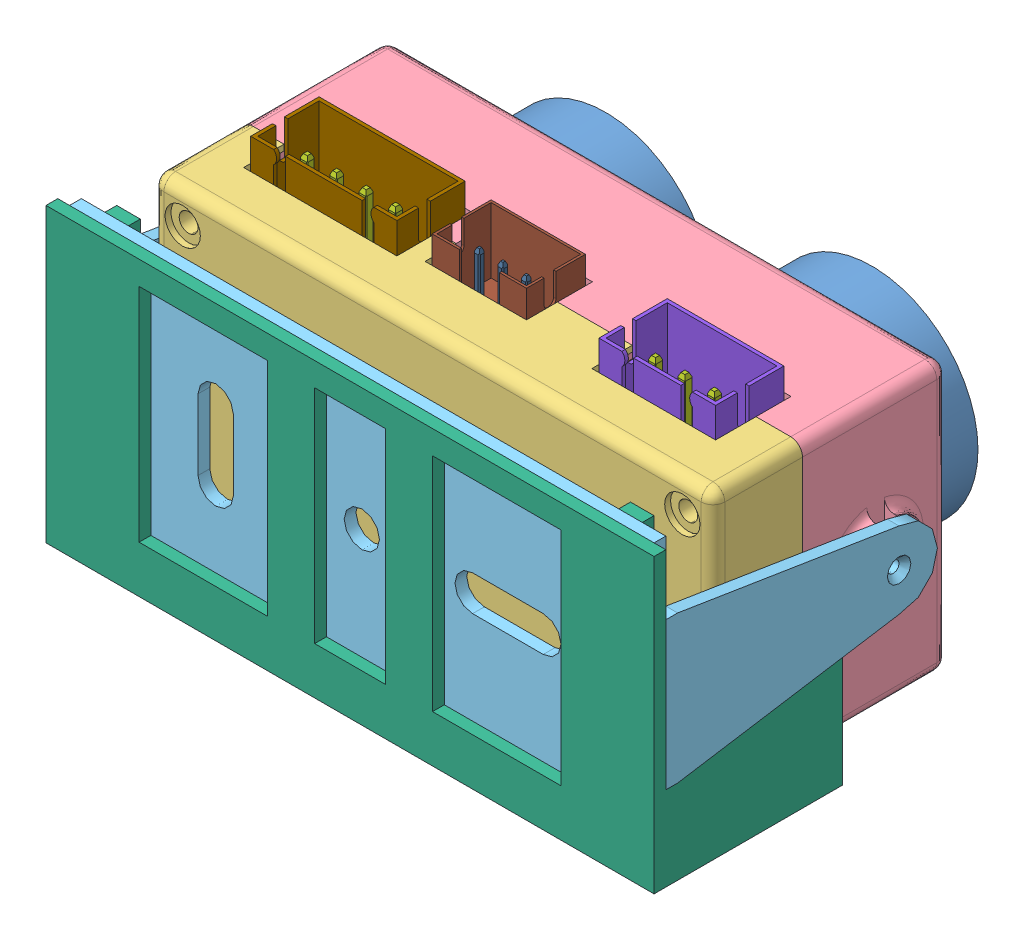
SolidWorks assembly assembly, configuration По умолчанию. Lengths in mm.
Overall size (51.6 27.1 32.99).
213 component instances, 60 part files, 18 mates.
Components (placement in the parent):
- hc-sr04-1: hc-sr04 [По умолчанию] at origin size (45.2 20.4 11.6)
- Assembly.step-1: Assembly.step [По умолчанию] at (-22.6 57.6501 -6.8032) x (1 0 0) z (0 0 1) size (47.6 23.9 18.81)
  - Assembly-asm1.step-1: Assembly-asm1.step [По умолчанию] at origin size (45.2 20.4 11.54)
    - Assembly-asm2.step-1: Assembly-asm2.step [По умолчанию] at (0 -47.4501 18.5211) x (1 0 0) z (0 0 -1) size (45.2 20.4 11.54)
      - X1.step-1: X1.step [По умолчанию] at (40.4891 10.7965 0) x (0 -1 0) z (0 0 1) size (10.16 2.54 11.54)
        - PLS-4.step-1: PLS-4.step [По умолчанию] at origin size (10.16 2.54 11.54)
          - PLS-1.step-1: PLS-1.step [По умолчанию] at (-1.27 0 0) size (2.54 2.54 11.54)
            - ____________.step-1: ____________.step [По умолчанию] at (0 0 -3) size (0.64 0.64 11.54)
            - _________.step-1: _________.step [По умолчанию] at origin size (2.54 2.54 2.54)
          - PLS-1.step-2: PLS-1.step [По умолчанию] at (-1.27 0 0) size (2.54 2.54 11.54)
            - ____________.step-1: ____________.step [По умолчанию] at (0 0 -3) size (0.64 0.64 11.54)
            - _________.step-1: _________.step [По умолчанию] at origin size (2.54 2.54 2.54)
          - PLS-1.step-3: PLS-1.step [По умолчанию] at (-3.81 0 0) size (2.54 2.54 11.54)
            - ____________.step-1: ____________.step [По умолчанию] at (0 0 -3) size (0.64 0.64 11.54)
            - _________.step-1: _________.step [По умолчанию] at origin size (2.54 2.54 2.54)
          - PLS-1.step-4: PLS-1.step [По умолчанию] at (1.27 0 0) size (2.54 2.54 11.54)
            - ____________.step-1: ____________.step [По умолчанию] at (0 0 -3) size (0.64 0.64 11.54)
            - _________.step-1: _________.step [По умолчанию] at origin size (2.54 2.54 2.54)
          - PLS-1.step-5: PLS-1.step [По умолчанию] at (3.81 0 0) size (2.54 2.54 11.54)
            - ____________.step-1: ____________.step [По умолчанию] at (0 0 -3) size (0.64 0.64 11.54)
            - _________.step-1: _________.step [По умолчанию] at origin size (2.54 2.54 2.54)
      - R4.step-1: R4.step [По умолчанию] at (17.4997 9.4504 0) x (1 0 0) z (0 0 1) size (1 0.51 0.35)
        - r0402.step-1: r0402.step [По умолчанию] at origin size (1 0.51 0.35)
      - R3.step-1: R3.step [По умолчанию] at (17.4997 6.8046 0) x (1 0 0) z (0 0 1) size (1 0.51 0.35)
        - r0402-0.step-1: r0402-0.step [По умолчанию] at origin size (1 0.51 0.35)
      - R2.step-1: R2.step [По умолчанию] at (17.4997 10.7046 0) x (-1 0 0) z (0 0 1) size (1 0.51 0.35)
        - r0402-1.step-1: r0402-1.step [По умолчанию] at origin size (1 0.51 0.35)
      - R1.step-1: R1.step [По умолчанию] at (17.4997 5.5504 0) x (-1 0 0) z (0 0 1) size (1 0.51 0.35)
        - r0402-2.step-1: r0402-2.step [По умолчанию] at origin size (1 0.51 0.35)
      - L1.step-1: L1.step [По умолчанию] at (32.2997 12.4504 0) x (0 -1 0) z (0 0 1) size (10.63 10.22 3.88)
        - Combine1.step-1: Combine1.step [По умолчанию] at origin size (10.63 10.22 3.88)
      - D1.step-1: D1.step [По умолчанию] at (23.1002 6.1507 0) x (-1 0 0) z (0 0 1) size (6 4.9 1.75)
        - User Library-SOIC-8-1.step-1: User Library-SOIC-8-1.step [По умолчанию] at origin size (6 4.9 1.75)
      - C7.step-1: C7.step [По умолчанию] at (17.4997 8.0804 0) x (-1 0 0) z (0 0 1) size (1 0.5 0.5)
        - User Library-Capacitor 0402.step-1: User Library-Capacitor 0402.step [По умолчанию] at origin size (1 0.5 0.5)
      - C6.step-1: C6.step [По умолчанию] at (17.4997 4.2457 0) x (1 0 0) z (0 0 1) size (1 0.5 0.5)
        - User Library-Capacitor 0402-3.step-1: User Library-Capacitor 0402-3.step [По умолчанию] at origin size (1 0.5 0.5)
      - C5.step-1: C5.step [По умолчанию] at (24.7543 14.1504 0) x (0 1 0) z (0 0 1) size (4 2.49 1.7)
        - User Library-1210(3225M) Cap.step-1: User Library-1210(3225M) Cap.step [По умолчанию] at origin size (4 2.49 1.7)
      - C4.step-1: C4.step [По умолчанию] at (21.2 14.15 0) x (0 1 0) z (0 0 1) size (4 2.49 1.7)
        - User Library-1210(3225M) Cap-4.step-1: User Library-1210(3225M) Cap-4.step [По умолчанию] at origin size (4 2.49 1.7)
      - C3.step-1: C3.step [По умолчанию] at (28.8 3.2 0) x (0 1 0) z (0 0 1) size (4 2.49 1.7)
        - User Library-1210(3225M) Cap-5.step-1: User Library-1210(3225M) Cap-5.step [По умолчанию] at origin size (4 2.49 1.7)
      - C2.step-1: C2.step [По умолчанию] at (17.4997 11.9589 0) x (-1 0 0) z (0 0 1) size (1 0.5 0.5)
        - User Library-Capacitor 0402-6.step-1: User Library-Capacitor 0402-6.step [По умолчанию] at origin size (1 0.5 0.5)
      - C1.step-1: C1.step [По умолчанию] at (33.9 4.9 0) x (0 -1 0) z (0 0 1) size (1 0.5 0.5)
        - User Library-Capacitor 0402-7.step-1: User Library-Capacitor 0402-7.step [По умолчанию] at origin size (1 0.5 0.5)
      - Board.step-1: Board.step [По умолчанию] at origin size (45.2 20.4 1.27)
  - Assembly-asm19.step-1: Assembly-asm19.step [По умолчанию] at origin size (47.6 23.9 18.21)
    - Assembly-asm20.step-1: Assembly-asm20.step [По умолчанию] at (0 -67.8501 12.5211) x (1 0 0) z (0 0 1) size (47.6 23.9 18.21)
      - C8.step-1: C8.step [По умолчанию] at (34.625 1.3 0) x (1 0 0) z (0 0 1) size (1 0.5 0.5)
        - User Library-Capacitor 0402-8.step-1: User Library-Capacitor 0402-8.step [По умолчанию] at origin size (1 0.5 0.5)
      - C7-1.step-1: C7-1.step [По умолчанию] at (32.625 1.3 0) x (-1 0 0) z (0 0 1) size (1 0.5 0.5)
        - User Library-Capacitor 0402-9.step-1: User Library-Capacitor 0402-9.step [По умолчанию] at origin size (1 0.5 0.5)
      - D4.step-1: D4.step [По умолчанию] at (33.625 4.8 0) x (0 1 0) z (0 0 1) size (4.3 4.5 1.51)
        - SW3dPS-SOT-89-1.step-1: SW3dPS-SOT-89-1.step [По умолчанию] at origin size (4.3 4.5 1.51)
      - X5.step-1: X5.step [По умолчанию] at (40.5 9.6 0) x (0 1 0) z (0 0 1) size (10.16 2.54 11.6)
        - User Library-PBS-04.step-1: User Library-PBS-04.step [По умолчанию] at origin size (10.16 2.54 11.6)
      - X6.step-1: X6.step [По умолчанию] at (24.1 1.9 0) x (-1 0 0) z (0 0 1) size (10.16 2.54 11.54)
        - PLS-4-1.step-1: PLS-4-1.step [По умолчанию] at origin size (10.16 2.54 11.54)
          - PLS-1.step-1: PLS-1.step [По умолчанию] at (-1.27 0 -1.2711) x (1 0 0) z (0 0 -1) size (2.54 2.54 11.54)
            - ____________.step-1: ____________.step [По умолчанию] at (0 0 -3) size (0.64 0.64 11.54)
            - _________.step-1: _________.step [По умолчанию] at origin size (2.54 2.54 2.54)
          - PLS-1.step-2: PLS-1.step [По умолчанию] at (-1.27 0 -1.2711) x (1 0 0) z (0 0 -1) size (2.54 2.54 11.54)
            - ____________.step-1: ____________.step [По умолчанию] at (0 0 -3) size (0.64 0.64 11.54)
            - _________.step-1: _________.step [По умолчанию] at origin size (2.54 2.54 2.54)
          - PLS-1.step-3: PLS-1.step [По умолчанию] at (-3.81 0 -1.2711) x (1 0 0) z (0 0 -1) size (2.54 2.54 11.54)
            - ____________.step-1: ____________.step [По умолчанию] at (0 0 -3) size (0.64 0.64 11.54)
            - _________.step-1: _________.step [По умолчанию] at origin size (2.54 2.54 2.54)
          - PLS-1.step-4: PLS-1.step [По умолчанию] at (1.27 0 -1.2711) x (1 0 0) z (0 0 -1) size (2.54 2.54 11.54)
            - ____________.step-1: ____________.step [По умолчанию] at (0 0 -3) size (0.64 0.64 11.54)
            - _________.step-1: _________.step [По умолчанию] at origin size (2.54 2.54 2.54)
          - PLS-1.step-5: PLS-1.step [По умолчанию] at (3.81 0 -1.2711) x (1 0 0) z (0 0 -1) size (2.54 2.54 11.54)
            - ____________.step-1: ____________.step [По умолчанию] at (0 0 -3) size (0.64 0.64 11.54)
            - _________.step-1: _________.step [По умолчанию] at origin size (2.54 2.54 2.54)
      - R1-1.step-1: R1-1.step [По умолчанию] at (6.2454 5.85 0) x (-1 0 0) z (0 0 1) size (1 0.51 0.35)
        - r0402-10.step-1: r0402-10.step [По умолчанию] at origin size (1 0.51 0.35)
      - C2-1.step-1: C2-1.step [По умолчанию] at (6.2454 2.35 0) x (1 0 0) z (0 0 1) size (1 0.5 0.5)
        - User Library-Capacitor 0402-11.step-1: User Library-Capacitor 0402-11.step [По умолчанию] at origin size (1 0.5 0.5)
      - C1-1.step-1: C1-1.step [По умолчанию] at (6.2454 4.817 0) x (1 0 0) z (0 0 1) size (1 0.5 0.5)
        - User Library-Capacitor 0402-12.step-1: User Library-Capacitor 0402-12.step [По умолчанию] at origin size (1 0.5 0.5)
      - X4.step-1: X4.step [По умолчанию] at (37.2 16.6 0) x (1 0 0) z (0 0 1) size (9.9 7.54 9.15)
        - xh-3aw.step-1: xh-3aw.step [По умолчанию] at origin size (9.9 7.54 9.15)
          - pin.step-1: pin.step [По умолчанию] at (-0.0001 0.02 -3.35) x (1 0 0) z (0 0 -1) size (0.64 6.32 7.12)
          - pin.step-2: pin.step [По умолчанию] at (-2.5001 0.02 -3.35) x (1 0 0) z (0 0 -1) size (0.64 6.32 7.12)
          - pin.step-3: pin.step [По умолчанию] at (2.4999 0.02 -3.35) x (1 0 0) z (0 0 -1) size (0.64 6.32 7.12)
          - xh-3aw-13.step-1: xh-3aw-13.step [По умолчанию] at origin size (9.9 7 5.8)
      - X3.step-1: X3.step [По умолчанию] at (8.9 16.7 0) x (1 0 0) z (0 0 1) size (12.4 7.54 9.15)
        - xh-4aw.step-1: xh-4aw.step [По умолчанию] at origin size (12.4 7.54 9.15)
          - pin.step-1: pin.step [По умолчанию] at (1.2501 -0.0199 -3.35) x (1 0 0) z (0 0 -1) size (0.64 6.32 7.12)
          - pin.step-2: pin.step [По умолчанию] at (3.7501 -0.0199 -3.35) x (1 0 0) z (0 0 -1) size (0.64 6.32 7.12)
          - pin.step-3: pin.step [По умолчанию] at (-3.7499 -0.0199 -3.35) x (1 0 0) z (0 0 -1) size (0.64 6.32 7.12)
          - pin.step-4: pin.step [По умолчанию] at (-1.2499 -0.0199 -3.35) x (1 0 0) z (0 0 -1) size (0.64 6.32 7.12)
          - xh-4aw-14.step-1: xh-4aw-14.step [По умолчанию] at origin size (12.4 7 5.8)
      - X2.step-1: X2.step [По умолчанию] at (21.3 17.6 0) x (1 0 0) z (0 0 1) size (8 6.25 8.4)
        - ph-3aw.step-1: ph-3aw.step [По умолчанию] at origin size (8 6.25 8.4)
          - pin-15.step-1: pin-15.step [По умолчанию] at (-2.0001 0.0249 -3.4) x (1 0 0) z (0 0 -1) size (0.5 5.25 6.65)
          - pin-15.step-2: pin-15.step [По умолчанию] at (1.9999 0.0249 -3.4) x (1 0 0) z (0 0 -1) size (0.5 5.25 6.65)
          - pin-15.step-3: pin-15.step [По умолчанию] at (-0.0001 0.0249 -3.4) x (1 0 0) z (0 0 -1) size (0.5 5.25 6.65)
          - ph-3aw-16.step-1: ph-3aw-16.step [По умолчанию] at origin size (8 6 5)
      - X1-1.step-1: X1-1.step [По умолчанию] at (3.5 5.835 0) x (0 1 0) z (0 0 1) size (5.08 6.09 4.74)
        - pls1.27-4R.step-1: pls1.27-4R.step [По умолчанию] at origin size (5.08 6.09 4.74)
          - housing.step-1: housing.step [По умолчанию] at (1.8951 0.5051 1.27) x (-1 0 0) z (0 1 0) size (1.27 2.4 1.5)
          - housing.step-2: housing.step [По умолчанию] at (-1.9149 0.5051 1.27) x (-1 0 0) z (0 1 0) size (1.27 2.4 1.5)
          - housing.step-3: housing.step [По умолчанию] at (-0.6449 0.5051 1.27) x (-1 0 0) z (0 1 0) size (1.27 2.4 1.5)
          - housing.step-4: housing.step [По умолчанию] at (0.6251 0.5051 1.27) x (-1 0 0) z (0 1 0) size (1.27 2.4 1.5)
          - pin-17.step-1: pin-17.step [По умолчанию] at (-0.6449 5.8951 1.27) x (-1 0 0) z (0 1 0) size (0.4 3.74 6.09)
          - pin-17.step-2: pin-17.step [По умолчанию] at (-1.9149 5.8951 1.27) x (-1 0 0) z (0 1 0) size (0.4 3.74 6.09)
          - pin-17.step-3: pin-17.step [По умолчанию] at (0.6251 5.8951 1.27) x (-1 0 0) z (0 1 0) size (0.4 3.74 6.09)
          - pin-17.step-4: pin-17.step [По умолчанию] at (1.8951 5.8951 1.27) x (-1 0 0) z (0 1 0) size (0.4 3.74 6.09)
      - VT3.step-1: VT3.step [По умолчанию] at (14.3043 13.2 0) x (0 1 0) z (0 0 1) size (2.64 3.05 1.12)
        - SOT95P237X112-3N.step.step-1: SOT95P237X112-3N.step.step [По умолчанию] at origin size (2.64 3.05 1.12)
          - Open CASCADE STEP translator 6.8 8.1.1.step-1: Open CASCADE STEP translator 6.8 8.1.1.step [По умолчанию] at (-0.7 -1.52 0) size (1.41 3.05 1.11)
          - Leader.step-1: Leader.step [По умолчанию] at (-0.7 -0.95 0) x (-1 0 0) z (0 0 1) size (0.62 0.5 0.61)
          - Leader.step-2: Leader.step [По умолчанию] at (-0.7 0.95 0) x (-1 0 0) z (0 0 1) size (0.62 0.5 0.61)
          - Leader.step-3: Leader.step [По умолчанию] at (0.7 0 0) size (0.62 0.5 0.61)
      - VT2.step-1: VT2.step [По умолчанию] at (10.2 13.2 0) x (0 1 0) z (0 0 1) size (2.64 3.05 1.12)
        - SOT95P237X112-3N.step-1.step-1: SOT95P237X112-3N.step-1.step [По умолчанию] at origin size (2.64 3.05 1.12)
          - Open CASCADE STEP translator 6.8 8.1.1.step-1: Open CASCADE STEP translator 6.8 8.1.1.step [По умолчанию] at (-0.7 -1.52 0) size (1.41 3.05 1.11)
          - Leader.step-1: Leader.step [По умолчанию] at (-0.7 -0.95 0) x (-1 0 0) z (0 0 1) size (0.62 0.5 0.61)
          - Leader.step-2: Leader.step [По умолчанию] at (-0.7 0.95 0) x (-1 0 0) z (0 0 1) size (0.62 0.5 0.61)
          - Leader.step-3: Leader.step [По умолчанию] at (0.7 0 0) size (0.62 0.5 0.61)
      - VT1.step-1: VT1.step [По умолчанию] at (6.0957 13.2 0) x (0 1 0) z (0 0 1) size (2.64 3.05 1.12)
        - SOT95P237X112-3N.step-2.step-1: SOT95P237X112-3N.step-2.step [По умолчанию] at origin size (2.64 3.05 1.12)
          - Open CASCADE STEP translator 6.8 8.1.1.step-1: Open CASCADE STEP translator 6.8 8.1.1.step [По умолчанию] at (-0.7 -1.52 0) size (1.41 3.05 1.11)
          - Leader.step-1: Leader.step [По умолчанию] at (-0.7 -0.95 0) x (-1 0 0) z (0 0 1) size (0.62 0.5 0.61)
          - Leader.step-2: Leader.step [По умолчанию] at (-0.7 0.95 0) x (-1 0 0) z (0 0 1) size (0.62 0.5 0.61)
          - Leader.step-3: Leader.step [По умолчанию] at (0.7 0 0) size (0.62 0.5 0.61)
      - VD1.step-1: VD1.step [По умолчанию] at (21.3 14.4 0) x (0 1 0) z (0 0 1) size (2.64 3.05 1.12)
        - SOT95P237X112-3N.step-3.step-1: SOT95P237X112-3N.step-3.step [По умолчанию] at origin size (2.64 3.05 1.12)
          - Open CASCADE STEP translator 6.8 8.1.1.step-1: Open CASCADE STEP translator 6.8 8.1.1.step [По умолчанию] at (-0.7 -1.52 0) size (1.41 3.05 1.11)
          - Leader.step-1: Leader.step [По умолчанию] at (-0.7 -0.95 0) x (-1 0 0) z (0 0 1) size (0.62 0.5 0.61)
          - Leader.step-2: Leader.step [По умолчанию] at (-0.7 0.95 0) x (-1 0 0) z (0 0 1) size (0.62 0.5 0.61)
          - Leader.step-3: Leader.step [По умолчанию] at (0.7 0 0) size (0.62 0.5 0.61)
      - R14.step-1: R14.step [По умолчанию] at (14.6085 10.0448 0) x (0 1 0) z (0 0 1) size (1 0.51 0.35)
        - r0402-18.step-1: r0402-18.step [По умолчанию] at origin size (1 0.51 0.35)
      - R13.step-1: R13.step [По умолчанию] at (13.3543 10.0448 0) x (0 1 0) z (0 0 1) size (1 0.51 0.35)
        - r0402-19.step-1: r0402-19.step [По умолчанию] at origin size (1 0.51 0.35)
      - R12.step-1: R12.step [По умолчанию] at (10.5043 10.0448 0) x (0 1 0) z (0 0 1) size (1 0.51 0.35)
        - r0402-20.step-1: r0402-20.step [По умолчанию] at origin size (1 0.51 0.35)
      - R11.step-1: R11.step [По умолчанию] at (9.25 10.0448 0) x (0 1 0) z (0 0 1) size (1 0.51 0.35)
        - r0402-21.step-1: r0402-21.step [По умолчанию] at origin size (1 0.51 0.35)
      - R10.step-1: R10.step [По умолчанию] at (6.4 10.0448 0) x (0 1 0) z (0 0 1) size (1 0.51 0.35)
        - r0402-22.step-1: r0402-22.step [По умолчанию] at origin size (1 0.51 0.35)
      - R9.step-1: R9.step [По умолчанию] at (5.1457 10.0448 0) x (0 1 0) z (0 0 1) size (1 0.51 0.35)
        - r0402-23.step-1: r0402-23.step [По умолчанию] at origin size (1 0.51 0.35)
      - R8.step-1: R8.step [По умолчанию] at (17.55 11.1 0) x (0 1 0) z (0 0 1) size (1 0.51 0.35)
        - r0402-24.step-1: r0402-24.step [По умолчанию] at origin size (1 0.51 0.35)
      - R7.step-1: R7.step [По умолчанию] at (18 4.817 0) x (1 0 0) z (0 0 1) size (1 0.51 0.35)
        - r0402-25.step-1: r0402-25.step [По умолчанию] at origin size (1 0.51 0.35)
      - R6.step-1: R6.step [По умолчанию] at (18 3.867 0) x (1 0 0) z (0 0 1) size (1 0.51 0.35)
        - r0402-26.step-1: r0402-26.step [По умолчанию] at origin size (1 0.51 0.35)
      - R5.step-1: R5.step [По умолчанию] at (20.3 10.6 0) x (1 0 0) z (0 0 1) size (1 0.51 0.35)
        - r0402-27.step-1: r0402-27.step [По умолчанию] at origin size (1 0.51 0.35)
      - R4-1.step-1: R4-1.step [По умолчанию] at (21.3 11.6707 0) x (1 0 0) z (0 0 1) size (1 0.51 0.35)
        - r0402-28.step-1: r0402-28.step [По умолчанию] at origin size (1 0.51 0.35)
      - R3-1.step-1: R3-1.step [По умолчанию] at (18 5.767 0) x (-1 0 0) z (0 0 1) size (1 0.51 0.35)
        - r0402-29.step-1: r0402-29.step [По умолчанию] at origin size (1 0.51 0.35)
      - R2-1.step-1: R2-1.step [По умолчанию] at (22.3 10.6 0) x (1 0 0) z (0 0 1) size (1 0.51 0.35)
        - r0402-30.step-1: r0402-30.step [По умолчанию] at origin size (1 0.51 0.35)
      - D3.step-1: D3.step [По умолчанию] at (33.625 12.17 0) x (0 1 0) z (0 0 1) size (4.3 4.5 1.51)
        - SW3dPS-SOT-89-1-31.step-1: SW3dPS-SOT-89-1-31.step [По умолчанию] at origin size (4.3 4.5 1.51)
      - D2.step-1: D2.step [По умолчанию] at (21.3 7.6 0) x (1 0 0) z (0 0 1) size (3.1 3.12 0.8)
        - User Library-My-DFN-8-3x3-0.5.step-1: User Library-My-DFN-8-3x3-0.5.step [По умолчанию] at origin size (3.1 3.12 0.8)
      - D1-1.step-1: D1-1.step [По умолчанию] at (10.8 4.1 0) x (1 0 0) z (0 0 1) size (5.12 5.12 0.6)
        - ufqfpn32.step-1: ufqfpn32.step [По умолчанию] at origin size (5.12 5.12 0.6)
          - pin-32.step-1: pin-32.step [По умолчанию] at (2.5601 0.2501 0) x (0 -1 0) z (0 0 1) size (0.28 0.51 0.15)
          - pin-32.step-2: pin-32.step [По умолчанию] at (-2.5599 -0.7499 0) x (0 1 0) z (0 0 1) size (0.28 0.51 0.15)
          - pin-32.step-3: pin-32.step [По умолчанию] at (-1.2499 2.5601 0) size (0.28 0.51 0.15)
          - pin-32.step-4: pin-32.step [По умолчанию] at (1.2501 -2.5599 0) x (-1 0 0) z (0 0 1) size (0.28 0.51 0.15)
          - pin-32.step-5: pin-32.step [По умолчанию] at (-0.7499 2.5601 0) size (0.28 0.51 0.15)
          - pin-32.step-6: pin-32.step [По умолчанию] at (1.2501 2.5601 0) size (0.28 0.51 0.15)
          - pin-32.step-7: pin-32.step [По умолчанию] at (2.5601 1.7501 0) x (0 -1 0) z (0 0 1) size (0.28 0.51 0.15)
          - pin-32.step-8: pin-32.step [По умолчанию] at (2.5601 -0.7499 0) x (0 -1 0) z (0 0 1) size (0.28 0.51 0.15)
          - pin-32.step-9: pin-32.step [По умолчанию] at (-2.5599 -0.2499 0) x (0 1 0) z (0 0 1) size (0.28 0.51 0.15)
          - pin-32.step-10: pin-32.step [По умолчанию] at (1.7501 -2.5599 0) x (-1 0 0) z (0 0 1) size (0.28 0.51 0.15)
          - pin-32.step-11: pin-32.step [По умолчанию] at (2.5601 0.7501 0) x (0 -1 0) z (0 0 1) size (0.28 0.51 0.15)
          - pin-32.step-12: pin-32.step [По умолчанию] at (-0.7499 -2.5599 0) x (-1 0 0) z (0 0 1) size (0.28 0.51 0.15)
          - pin-32.step-13: pin-32.step [По умолчанию] at (-0.2499 2.5601 0) size (0.28 0.51 0.15)
          - pin-32.step-14: pin-32.step [По умолчанию] at (2.5601 1.2501 0) x (0 -1 0) z (0 0 1) size (0.28 0.51 0.15)
          - pin-32.step-15: pin-32.step [По умолчанию] at (0.7501 -2.5599 0) x (-1 0 0) z (0 0 1) size (0.28 0.51 0.15)
          - pin-32.step-16: pin-32.step [По умолчанию] at (-2.5599 -1.7499 0) x (0 1 0) z (0 0 1) size (0.28 0.51 0.15)
          - pin-32.step-17: pin-32.step [По умолчанию] at (1.7501 2.5601 0) size (0.28 0.51 0.15)
          - pin-32.step-18: pin-32.step [По умолчанию] at (2.5601 -0.2499 0) x (0 -1 0) z (0 0 1) size (0.28 0.51 0.15)
          - pin-32.step-19: pin-32.step [По умолчанию] at (-1.2499 -2.5599 0) x (-1 0 0) z (0 0 1) size (0.28 0.51 0.15)
          - pin-32.step-20: pin-32.step [По умолчанию] at (0.2501 2.5601 0) size (0.28 0.51 0.15)
          - pin-32.step-21: pin-32.step [По умолчанию] at (-2.5599 1.7501 0) x (0 1 0) z (0 0 1) size (0.28 0.51 0.15)
          - pin-32.step-22: pin-32.step [По умолчанию] at (0.2501 -2.5599 0) x (-1 0 0) z (0 0 1) size (0.28 0.51 0.15)
          - pin-32.step-23: pin-32.step [По умолчанию] at (-0.2499 -2.5599 0) x (-1 0 0) z (0 0 1) size (0.28 0.51 0.15)
          - pin-32.step-24: pin-32.step [По умолчанию] at (-2.5599 0.7501 0) x (0 1 0) z (0 0 1) size (0.28 0.51 0.15)
          - pin-32.step-25: pin-32.step [По умолчанию] at (2.5601 -1.2499 0) x (0 -1 0) z (0 0 1) size (0.28 0.51 0.15)
          - pad.step-1: pad.step [По умолчанию] at (-0.0001 0.0001 0.152) x (0 1 0) z (0 0 -1) size (3.6 3.6 0.15)
          - pin-32.step-26: pin-32.step [По умолчанию] at (0.7501 2.5601 0) size (0.28 0.51 0.15)
          - pin-32.step-27: pin-32.step [По умолчанию] at (-2.5599 1.2501 0) x (0 1 0) z (0 0 1) size (0.28 0.51 0.15)
          - pin-32.step-28: pin-32.step [По умолчанию] at (-1.7499 2.5601 0) size (0.28 0.51 0.15)
          - pin-32.step-29: pin-32.step [По умолчанию] at (-2.5599 -1.2499 0) x (0 1 0) z (0 0 1) size (0.28 0.51 0.15)
          - pin-32.step-30: pin-32.step [По умолчанию] at (-2.5599 0.2501 0) x (0 1 0) z (0 0 1) size (0.28 0.51 0.15)
          - pin-32.step-31: pin-32.step [По умолчанию] at (2.5601 -1.7499 0) x (0 -1 0) z (0 0 1) size (0.28 0.51 0.15)
          - pin-32.step-32: pin-32.step [По умолчанию] at (-1.7499 -2.5599 0) x (-1 0 0) z (0 0 1) size (0.28 0.51 0.15)
          - ufqfpn32-33.step-1: ufqfpn32-33.step [По умолчанию] at origin size (5.1 5.1 0.6)
      - C6-1.step-1: C6-1.step [По умолчанию] at (32.625 8.57 0) x (-1 0 0) z (0 0 1) size (1 0.5 0.5)
        - User Library-Capacitor 0402-34.step-1: User Library-Capacitor 0402-34.step [По умолчанию] at origin size (1 0.5 0.5)
      - C5-1.step-1: C5-1.step [По умолчанию] at (34.625 8.57 0) x (1 0 0) z (0 0 1) size (1 0.5 0.5)
        - User Library-Capacitor 0402-35.step-1: User Library-Capacitor 0402-35.step [По умолчанию] at origin size (1 0.5 0.5)
      - C4-1.step-1: C4-1.step [По умолчанию] at (18.45 11.1 0) x (0 1 0) z (0 0 1) size (1 0.5 0.5)
        - User Library-Capacitor 0402-36.step-1: User Library-Capacitor 0402-36.step [По умолчанию] at origin size (1 0.5 0.5)
      - C3-1.step-1: C3-1.step [По умолчанию] at (19.05 8.5 0) x (0 1 0) z (0 0 1) size (1 0.5 0.5)
        - User Library-Capacitor 0402-37.step-1: User Library-Capacitor 0402-37.step [По умолчанию] at origin size (1 0.5 0.5)
      - Board-38.step-1: Board-38.step [По умолчанию] at origin size (45.2 20.4 1.27)
- bottom case-1: bottom case [По умолчанию] at (-22.6 -10.2 11.7179) x (1 0 0) z (0 -1 0) size (47.6 7.6 22.8)
- top case-1: top case [По умолчанию] at (-22.6 -10.2 8.389) x (-1 0 0) z (0 0 -1) size (49.6 22.8 13.39)
- holder-1: holder [По умолчанию] at (-22.6 -10.2 15.989) x (1 0 0) z (0 0 1) size (51.6 22.9 23.04)
- cover-spacer-1: cover-spacer [По умолчанию] at (-22.6 -10.2 21.989) x (1 0 0) z (0 0 1) size (51.6 24.8 16)
Mates (geometry in assembly coordinates):
- Концентричный1: concentric: cylinder of hc-sr04-1 through (-21.2 -8.7 0) axis (0 0 1) radius 1; cylinder of Assembly.step-1/Assembly-asm19.step-1/Assembly-asm20.step-1/Board-38.step-1 through (-21.2 -8.7 4.4468) axis (0 0 1) radius 0.9055
- Концентричный2: concentric: cylinder of hc-sr04-1 through (21.2 -8.7 0) axis (0 0 1) radius 1; circle of Assembly.step-1/Assembly-asm19.step-1/Assembly-asm20.step-1/Board-38.step-1
- На месте1: in place: plane of Assembly.step-1/Assembly-asm1.step-1/Assembly-asm2.step-1/Board.step-1 through (22.6 -10.2 12.989) normal (0 -1 0); plane of ? through (0 -10.2 0) normal (0 -1 0); moOrthogonalPlaneRef_w of Assembly.step-1/Assembly-asm1.step-1/Assembly-asm2.step-1/Board.step-1 through (22.6 -10.2 12.989) normal (0 -1 0); plane of ? through (0 -10.2 0) normal (0 0 -1); plane of Assembly.step-1/Assembly-asm1.step-1/Assembly-asm2.step-1/Board.step-1 through (22.6 -10.2 12.989) normal (0 -1 0); plane of ? through (0 -10.2 0) normal (-1 0 0); plane of Assembly.step-1/Assembly-asm1.step-1/Assembly-asm2.step-1/Board.step-1 through (22.6 -10.2 12.989) normal (0 -1 0); unknown of bottom case-1
- Совпадение3: coincident: plane of Assembly.step-1/Assembly-asm1.step-1/Assembly-asm2.step-1/Board.step-1; plane of bottom case-1
- Совпадение4: coincident: moOrthogonalPlaneRef_w of Assembly.step-1/Assembly-asm1.step-1/Assembly-asm2.step-1/Board.step-1 through (-22.6 -10.2 11.7179) normal (0 0 1); plane of bottom case-1 through (-22.6 -10.2 11.7179) normal (0 0 1)
- Совпадение5: coincident: moOrthogonalPlaneRef_w of Assembly.step-1/Assembly-asm1.step-1/Assembly-asm2.step-1/Board.step-1 through (-22.6 -10.2 11.7179) normal (-1 0 0); plane of bottom case-1 through (-22.6 -10.2 11.7179) normal (1 0 0)
- На месте2: in place: plane of bottom case-1 through (-22.6 -10.2 8.389) normal (0 0 -1); plane of ? through (0 0 8.389) normal (0 0 -1); plane of bottom case-1 through (-22.6 -10.2 8.389) normal (0 0 -1); plane of ? through (0 0 8.389) normal (0 1 0); plane of bottom case-1 through (-22.6 -10.2 8.389) normal (0 0 -1); plane of ? through (0 0 8.389) normal (-1 0 0); plane of bottom case-1 through (-22.6 -10.2 8.389) normal (0 0 -1); unknown of top case-1
- Совпадение6: coincident: plane of bottom case-1; plane of top case-1
- Совпадение7: coincident: moOrthogonalPlaneRef_w of bottom case-1 through (-22.6 -10.2 8.389) normal (0 1 0); plane of top case-1 through (-22.6 -10.2 8.389) normal (0 1 0)
- Совпадение8: coincident: moOrthogonalPlaneRef_w of bottom case-1 through (-22.6 -10.2 8.389) normal (1 0 0); plane of top case-1 through (-22.6 -10.2 8.389) normal (-1 0 0)
- На месте3: in place: plane of bottom case-1 through (-22.6 -10.2 15.989) normal (0 0 1); plane of ? through (0 0 15.989) normal (0 0 1); plane of bottom case-1 through (-22.6 -10.2 15.989) normal (0 0 1); plane of ? through (0 0 15.989) normal (0 1 0); plane of bottom case-1 through (-22.6 -10.2 15.989) normal (0 0 1); plane of ? through (0 0 15.989) normal (1 0 0); plane of bottom case-1 through (-22.6 -10.2 15.989) normal (0 0 1); unknown of holder-1
- Совпадение1: coincident: plane of bottom case-1; plane of holder-1
- Совпадение2: coincident: moOrthogonalPlaneRef_w of bottom case-1 through (-22.6 -10.2 15.989) normal (0 1 0); plane of holder-1 through (-22.6 -10.2 15.989) normal (0 1 0)
- Совпадение3: coincident: moOrthogonalPlaneRef_w of bottom case-1 through (-22.6 -10.2 15.989) normal (-1 0 0); plane of holder-1 through (-22.6 -10.2 15.989) normal (1 0 0)
- На месте4: in place: plane of holder-1 through (-22.6 -10.2 21.989) normal (0 0 1); plane of ? through (0 0 21.989) normal (0 0 1); plane of holder-1 through (-22.6 -10.2 21.989) normal (0 0 1); plane of ? through (0 0 21.989) normal (0 1 0); plane of holder-1 through (-22.6 -10.2 21.989) normal (0 0 1); plane of ? through (0 0 21.989) normal (1 0 0); plane of holder-1 through (-22.6 -10.2 21.989) normal (0 0 1); unknown of cover-spacer-1
- Совпадение1: coincident: plane of holder-1; plane of cover-spacer-1
- Совпадение2: coincident: moOrthogonalPlaneRef_w of holder-1 through (-22.6 -10.2 21.989) normal (0 1 0); plane of cover-spacer-1 through (-22.6 -10.2 21.989) normal (0 1 0)
- Совпадение3: coincident: moOrthogonalPlaneRef_w of holder-1 through (-22.6 -10.2 21.989) normal (-1 0 0); plane of cover-spacer-1 through (-22.6 -10.2 21.989) normal (1 0 0)
